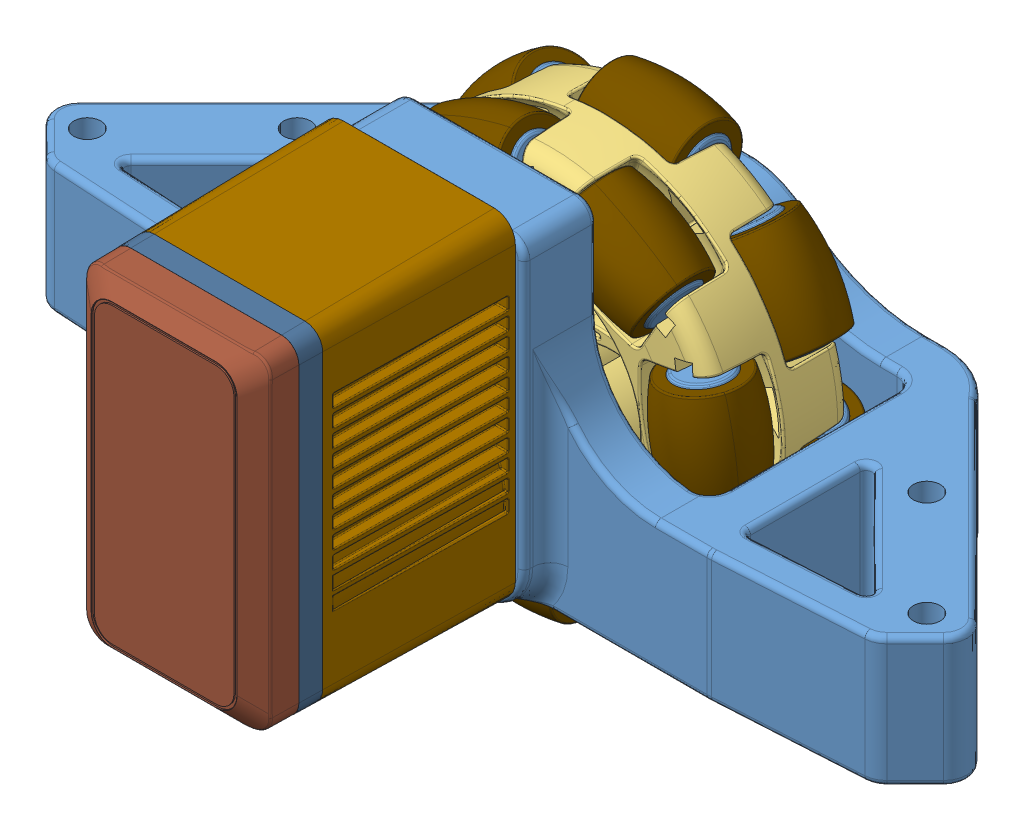
SolidWorks assembly holo_bracket_v4_testfit, configuration Default. Lengths in mm.
Overall size (155.99 97.03 100.21).
88 component instances, 22 part files, 14 mates.
Components (placement in the parent):
- holo_bracket_v4-1: holo_bracket_v4 [Default] at (53.3418 73.7776 128.0643) size (155.99 57.17 55.6)
- V5 Smart Motor (276-4840) no cap-1: V5 Smart Motor (276-4840) no cap [Default] at (53.3418 105.5276 175.3143) x (0 -1 0) z (0 0 -1) size (59.01 35.33 59.91)
  - V5 Smart Motor (276-4840).step-1: V5 Smart Motor (276-4840).step [Default] at origin size (59.01 35.33 59.91)
    - 276-4840-900 Rev6_Instruction.step-1: 276-4840-900 Rev6_Instruction.step [Default] at (-14.3 0 -17.2) size (52.79 15.94 38.15)
      - 276-4840-901 Rev6.step-1: 276-4840-901 Rev6.step [Default] at (10.75 -10.05 17.8) x (-1 0 0) z (0 0 1) size (49.9 1.6 38.15)
      - 276-4840-902 Rev2.step-1: 276-4840-902 Rev2.step [Default] at (31.25 -9.25 6.2) x (0 0 -1) z (0 -1 0) size (10.35 11.39 15.94)
      - 276-4840-022 Rev4.step-1: 276-4840-022 Rev4.step [Default] at (31.25 -9.25 6.2) x (0 0 -1) z (1 0 0) size (10.26 9.1 5.51)
    - 276-4840-110 Rev10_Instruction.step-1: 276-4840-110 Rev10_Instruction.step [Default] at (12.7 0 14.7) size (35.33 35.33 31.1)
      - 276-4840-061 Rev7_Ring_Gear_Fixed01 .6 Rev3.step-1: 276-4840-061 Rev7_Ring_Gear_Fixed01 .6 Rev3.step [Default] at origin size (28.79 28.39 24.6)
      - 276-4840-018 Rev6.step-1: 276-4840-018 Rev6.step [Default] at (0 0 6.7) x (-0.483174 0.875524 0) z (0 0 1) size (26 26 12.3)
      - 276-4840-059 Rev2.step-1: 276-4840-059 Rev2.step [Default] at (0 0 10.3) size (28.4 28.4 8.5)
      - 276-4840-062 Rev1.step-1: 276-4840-062 Rev1.step [Default] at (-12.1353 8.8168 12.3) x (0.956835 -0.290632 0) z (-0.290632 -0.956835 0) size (3.2 6.56 3.2)
      - 276-4840-062 Rev1.step-2: 276-4840-062 Rev1.step [Default] at (12.1353 8.8168 12.3) x (0.978427 0.206591 0) z (0.206591 -0.978427 0) size (3.2 6.56 3.2)
      - 276-4840-062 Rev1.step-3: 276-4840-062 Rev1.step [Default] at (-12.1353 -8.8168 12.3) x (0.72563 0.688086 0) z (0.688086 -0.72563 0) size (3.2 6.56 3.2)
    - 276-4840-001 Rev38.step-1: 276-4840-001 Rev38.step [Default] at origin size (57.3 33 46.9)
    - 276-4840-005 Rev27.step-1: 276-4840-005 Rev27.step [Default] at (0 0 -17.95) size (56.17 31.87 12.9)
    - 276-4840-004 Rev16.step-1: 276-4840-004 Rev16.step [Default] at (0 0 -19.2) size (56.01 31.71 9.21)
    - 276-4840-009 Rev3.step-1: 276-4840-009 Rev3.step [Default] at (25.45 13.5 15.7) x (0.19987 -0.979823 0) z (-0.979823 -0.19987 0) size (3.4 41.31 4.34)
    - 276-4840-009 Rev3.step-2: 276-4840-009 Rev3.step [Default] at (-25.45 -13.5 15.7) x (-0.998855 0.047836 0) z (0.047836 0.998855 0) size (3.4 41.31 4.34)
    - 276-4840-009 Rev3.step-3: 276-4840-009 Rev3.step [Default] at (25.45 -13.5 15.7) x (-0.975374 0.220559 0) z (0.220559 0.975374 0) size (3.4 41.31 4.34)
    - 276-4840-009 Rev3.step-4: 276-4840-009 Rev3.step [Default] at (-25.45 13.5 15.7) x (-0.922256 0.38658 0) z (0.38658 0.922256 0) size (3.4 41.31 4.34)
    - 276-4840-025 Rev19.step-1: 276-4840-025 Rev19.step [Default] at (12.7 0 -22.63) x (-0.993315 0.115437 0) z (0 0 1) size (14.82 14.83 35.18)
- 0.375_ ID x 0.875_ OD x 0.281_ WD (Radial Bearing) (217-3239)-1: 0.375_ ID x 0.875_ OD x 0.281_ WD (Radial Bearing) (217-3239) [Default] at (53.3418 92.8276 103.3769) x (0 0 1) z (-1 0 0) size (7.14 22.23 22.23)
- 0.375in_ID_Bearing_Insert-1: 0.375in_ID_Bearing_Insert [Default] at (53.3418 92.8276 110.5143) x (-0.838817 0.544413 0) z (0 0 -1) size (9.4 9.4 7.14)
- Drive Shaft 2in-1: Drive Shaft 2in [Default] at (53.3418 92.8276 1.1143) x (-0.544413 -0.838817 0) z (0 0 1) size (3.28 3.28 50.8)
- Shaft Collar (276-2010)-1: Shaft Collar (276-2010) [Default] at (53.3418 92.8276 113.8163) size (11 11.35 6.6)
- 2.75 Omni with inserts (276-1902) -1: 2.75 Omni with inserts (276-1902)  [Default] at (0.1559 110.7488 59.7876) x (0.152128 -0.988361 0) z (0 0 1) size (87.15 87.98 47.75)
  - 2.75 Omni-Directional Wheel - Double Roller (276-1902) -1: 2.75 Omni-Directional Wheel - Double Roller (276-1902)  [Default] at (25.8037 49.8406 68.5807) size (87.15 87.98 47.75)
    - 2.75 Omni-Directional Wheel - Double Roller (276-1902) .step-1: 2.75 Omni-Directional Wheel - Double Roller (276-1902) .step [Default] at origin size (87.15 87.98 47.75)
      - 276-1902-010 Rev1.step-1: 276-1902-010 Rev1.step [Default] at (0 27.5 8) x (1 0 0) z (0 0.828233 0.560383) size (23 27.81 20.35)
        - 276-1902-011 Rev1.step-1: 276-1902-011 Rev1.step [Default] at (0 -6.325 -26.7627) x (1 0 0) z (0 -0.973191 0.23) size (16.5 15 25.03)
        - 276-1902-012 Rev1.step-1: 276-1902-012 Rev1.step [Default] at origin size (17.5 10.34 18.34)
        - 276-1902-003 Rev1.step-1: 276-1902-003 Rev1.step [Default] x (0 -0.928523 0.371275) z (1 0 0) size (2 2 23)
      - 276-1902-010 Rev1.step-2: 276-1902-010 Rev1.step [Default] at (0 -27.5 -8) x (1 0 0) z (0 0.410464 0.911877) size (23 27.81 20.35)
        - 276-1902-011 Rev1.step-1: 276-1902-011 Rev1.step [Default] at (0 -6.325 -26.7627) x (1 0 0) z (0 -0.973191 0.23) size (16.5 15 25.03)
        - 276-1902-012 Rev1.step-1: 276-1902-012 Rev1.step [Default] at origin size (17.5 10.34 18.34)
        - 276-1902-003 Rev1.step-1: 276-1902-003 Rev1.step [Default] x (0 -0.928523 0.371275) z (1 0 0) size (2 2 23)
      - 276-1902-010 Rev1.step-3: 276-1902-010 Rev1.step [Default] at (-21.5004 -17.146 -8) x (0.62349 -0.781831 0) z (0.320913 0.25592 0.911877) size (23 27.81 20.35)
        - 276-1902-011 Rev1.step-1: 276-1902-011 Rev1.step [Default] at (0 -6.325 -26.7627) x (1 0 0) z (0 -0.973191 0.23) size (16.5 15 25.03)
        - 276-1902-012 Rev1.step-1: 276-1902-012 Rev1.step [Default] at origin size (17.5 10.34 18.34)
        - 276-1902-003 Rev1.step-1: 276-1902-003 Rev1.step [Default] x (0 -0.928523 0.371275) z (1 0 0) size (2 2 23)
      - 276-1902-010 Rev1.step-4: 276-1902-010 Rev1.step [Default] at (-26.8105 6.1193 -8) x (-0.222521 -0.974928 0) z (0.400172 -0.091337 0.911877) size (23 27.81 20.35)
        - 276-1902-011 Rev1.step-1: 276-1902-011 Rev1.step [Default] at (0 -6.325 -26.7627) x (1 0 0) z (0 -0.973191 0.23) size (16.5 15 25.03)
        - 276-1902-012 Rev1.step-1: 276-1902-012 Rev1.step [Default] at origin size (17.5 10.34 18.34)
        - 276-1902-003 Rev1.step-1: 276-1902-003 Rev1.step [Default] x (0 -0.928523 0.371275) z (1 0 0) size (2 2 23)
      - 276-1902-010 Rev1.step-5: 276-1902-010 Rev1.step [Default] at (-11.9318 24.7766 -8) x (-0.900969 -0.433884 0) z (0.178093 -0.369815 0.911877) size (23 27.81 20.35)
        - 276-1902-011 Rev1.step-1: 276-1902-011 Rev1.step [Default] at (0 -6.325 -26.7627) x (1 0 0) z (0 -0.973191 0.23) size (16.5 15 25.03)
        - 276-1902-012 Rev1.step-1: 276-1902-012 Rev1.step [Default] at origin size (17.5 10.34 18.34)
        - 276-1902-003 Rev1.step-1: 276-1902-003 Rev1.step [Default] x (0 -0.928523 0.371275) z (1 0 0) size (2 2 23)
      - 276-1902-010 Rev1.step-6: 276-1902-010 Rev1.step [Default] at (11.9318 24.7766 -8) x (-0.900969 0.433884 0) z (-0.178093 -0.369815 0.911877) size (23 27.81 20.35)
        - 276-1902-011 Rev1.step-1: 276-1902-011 Rev1.step [Default] at (0 -6.325 -26.7627) x (1 0 0) z (0 -0.973191 0.23) size (16.5 15 25.03)
        - 276-1902-012 Rev1.step-1: 276-1902-012 Rev1.step [Default] at origin size (17.5 10.34 18.34)
        - 276-1902-003 Rev1.step-1: 276-1902-003 Rev1.step [Default] x (0 -0.928523 0.371275) z (1 0 0) size (2 2 23)
      - 276-1902-010 Rev1.step-7: 276-1902-010 Rev1.step [Default] at (26.8105 6.1193 -8) x (-0.222521 0.974928 0) z (-0.400172 -0.091337 0.911877) size (23 27.81 20.35)
        - 276-1902-011 Rev1.step-1: 276-1902-011 Rev1.step [Default] at (0 -6.325 -26.7627) x (1 0 0) z (0 -0.973191 0.23) size (16.5 15 25.03)
        - 276-1902-012 Rev1.step-1: 276-1902-012 Rev1.step [Default] at origin size (17.5 10.34 18.34)
        - 276-1902-003 Rev1.step-1: 276-1902-003 Rev1.step [Default] x (0 -0.928523 0.371275) z (1 0 0) size (2 2 23)
      - 276-1902-010 Rev1.step-8: 276-1902-010 Rev1.step [Default] at (21.5004 -17.146 -8) x (0.62349 0.781831 0) z (-0.320913 0.25592 0.911877) size (23 27.81 20.35)
        - 276-1902-011 Rev1.step-1: 276-1902-011 Rev1.step [Default] at (0 -6.325 -26.7627) x (1 0 0) z (0 -0.973191 0.23) size (16.5 15 25.03)
        - 276-1902-012 Rev1.step-1: 276-1902-012 Rev1.step [Default] at origin size (17.5 10.34 18.34)
        - 276-1902-003 Rev1.step-1: 276-1902-003 Rev1.step [Default] x (0 -0.928523 0.371275) z (1 0 0) size (2 2 23)
      - 276-1902-010 Rev1.step-9: 276-1902-010 Rev1.step [Default] at (21.5004 17.146 8) x (0.62349 -0.781831 0) z (0.647539 0.516395 0.560383) size (23 27.81 20.35)
        - 276-1902-011 Rev1.step-1: 276-1902-011 Rev1.step [Default] at (0 -6.325 -26.7627) x (1 0 0) z (0 -0.973191 0.23) size (16.5 15 25.03)
        - 276-1902-012 Rev1.step-1: 276-1902-012 Rev1.step [Default] at origin size (17.5 10.34 18.34)
        - 276-1902-003 Rev1.step-1: 276-1902-003 Rev1.step [Default] x (0 -0.928523 0.371275) z (1 0 0) size (2 2 23)
      - 276-1902-010 Rev1.step-10: 276-1902-010 Rev1.step [Default] at (26.8105 -6.1193 8) x (-0.222521 -0.974928 0) z (0.807468 -0.184299 0.560383) size (23 27.81 20.35)
        - 276-1902-011 Rev1.step-1: 276-1902-011 Rev1.step [Default] at (0 -6.325 -26.7627) x (1 0 0) z (0 -0.973191 0.23) size (16.5 15 25.03)
        - 276-1902-012 Rev1.step-1: 276-1902-012 Rev1.step [Default] at origin size (17.5 10.34 18.34)
        - 276-1902-003 Rev1.step-1: 276-1902-003 Rev1.step [Default] x (0 -0.928523 0.371275) z (1 0 0) size (2 2 23)
      - 276-1902-010 Rev1.step-11: 276-1902-010 Rev1.step [Default] at (11.9318 -24.7766 8) x (-0.900969 -0.433884 0) z (0.359357 -0.746212 0.560383) size (23 27.81 20.35)
        - 276-1902-011 Rev1.step-1: 276-1902-011 Rev1.step [Default] at (0 -6.325 -26.7627) x (1 0 0) z (0 -0.973191 0.23) size (16.5 15 25.03)
        - 276-1902-012 Rev1.step-1: 276-1902-012 Rev1.step [Default] at origin size (17.5 10.34 18.34)
        - 276-1902-003 Rev1.step-1: 276-1902-003 Rev1.step [Default] x (0 -0.928523 0.371275) z (1 0 0) size (2 2 23)
      - 276-1902-010 Rev1.step-12: 276-1902-010 Rev1.step [Default] at (-11.9318 -24.7766 8) x (-0.900969 0.433884 0) z (-0.359357 -0.746212 0.560383) size (23 27.81 20.35)
        - 276-1902-011 Rev1.step-1: 276-1902-011 Rev1.step [Default] at (0 -6.325 -26.7627) x (1 0 0) z (0 -0.973191 0.23) size (16.5 15 25.03)
        - 276-1902-012 Rev1.step-1: 276-1902-012 Rev1.step [Default] at origin size (17.5 10.34 18.34)
        - 276-1902-003 Rev1.step-1: 276-1902-003 Rev1.step [Default] x (0 -0.928523 0.371275) z (1 0 0) size (2 2 23)
      - 276-1902-010 Rev1.step-13: 276-1902-010 Rev1.step [Default] at (-26.8105 -6.1193 8) x (-0.222521 0.974928 0) z (-0.807468 -0.184299 0.560383) size (23 27.81 20.35)
        - 276-1902-011 Rev1.step-1: 276-1902-011 Rev1.step [Default] at (0 -6.325 -26.7627) x (1 0 0) z (0 -0.973191 0.23) size (16.5 15 25.03)
        - 276-1902-012 Rev1.step-1: 276-1902-012 Rev1.step [Default] at origin size (17.5 10.34 18.34)
        - 276-1902-003 Rev1.step-1: 276-1902-003 Rev1.step [Default] x (0 -0.928523 0.371275) z (1 0 0) size (2 2 23)
      - 276-1902-010 Rev1.step-14: 276-1902-010 Rev1.step [Default] at (-21.5004 17.146 8) x (0.62349 0.781831 0) z (-0.647539 0.516395 0.560383) size (23 27.81 20.35)
        - 276-1902-011 Rev1.step-1: 276-1902-011 Rev1.step [Default] at (0 -6.325 -26.7627) x (1 0 0) z (0 -0.973191 0.23) size (16.5 15 25.03)
        - 276-1902-012 Rev1.step-1: 276-1902-012 Rev1.step [Default] at origin size (17.5 10.34 18.34)
        - 276-1902-003 Rev1.step-1: 276-1902-003 Rev1.step [Default] x (0 -0.928523 0.371275) z (1 0 0) size (2 2 23)
      - 276-1902-002 Rev3.step-1: 276-1902-002 Rev3.step [Default] at origin size (66.55 66.02 25.07)
  - Metal Shaft Inserts (276-3881-002)-1: Metal Shaft Inserts (276-3881-002) [Default] at (25.8037 49.8406 79.8307) x (0 -1 0) z (1 0 0) size (10.03 5.08 10.03)
  - Metal Shaft Inserts (276-3881-002)-2: Metal Shaft Inserts (276-3881-002) [Default] at (25.8037 49.8406 57.3307) x (1 0 0) z (0 -1 0) size (10.03 5.08 10.03)
Mates (geometry in assembly coordinates):
- Concentric1: concentric aligned: cylinder of holo_bracket_v4-1 through (53.3418 92.8276 102.5133) axis (0 0 1) radius 14.5; cone of V5 Smart Motor (276-4840) no cap-1/V5 Smart Motor (276-4840).step-1/276-4840-110 Rev10_Instruction.step-1/276-4840-061 Rev7_Ring_Gear_Fixed01 .6 Rev3.step-1 through (53.3418 92.8276 172.9143) axis (0 0 1)
- Coincident1: coincident anti-aligned: plane of holo_bracket_v4-1 through (53.3418 73.7776 158.1143) normal (0 0 1); plane of V5 Smart Motor (276-4840) no cap-1/V5 Smart Motor (276-4840).step-1/276-4840-001 Rev38.step-1 through (40.4418 130.5776 158.1143) normal (0 0 -1)
- Parallel1: parallel aligned: line of holo_bracket_v4-1 through (39.3418 130.4776 157.1143) axis (1 0 0); line of V5 Smart Motor (276-4840) no cap-1/V5 Smart Motor (276-4840).step-1/276-4840-001 Rev38.step-1 through (40.4418 134.1776 159.1143) axis (1 0 0)
- Concentric2: concentric anti-aligned: cylinder of 0.375_ ID x 0.875_ OD x 0.281_ WD (Radial Bearing) (217-3239)-1 through (53.3418 92.8276 88.84) axis (0 0 -1) radius 4.763; cylinder of 0.375in_ID_Bearing_Insert-1 through (53.3418 92.8276 103.3769) axis (0 0 1) radius 4.7
- Coincident2: coincident aligned: plane of 0.375_ ID x 0.875_ OD x 0.281_ WD (Radial Bearing) (217-3239)-1 through (53.3418 87.6646 103.3769) normal (0 0 -1); plane of 0.375in_ID_Bearing_Insert-1 through (53.3418 92.8276 103.3769) normal (0 0 -1)
- Concentric3: concentric anti-aligned: cylinder of holo_bracket_v4-1 through (53.3418 92.8276 103.3769) axis (0 0 1) radius 11.25; cylinder of 0.375_ ID x 0.875_ OD x 0.281_ WD (Radial Bearing) (217-3239)-1 through (53.3418 92.8276 88.84) axis (0 0 -1) radius 11.113
- Coincident3: coincident anti-aligned: plane of holo_bracket_v4-1 through (53.3418 92.8276 103.3769) normal (0 0 1); plane of 0.375_ ID x 0.875_ OD x 0.281_ WD (Radial Bearing) (217-3239)-1 through (53.3418 83.3446 103.3769) normal (0 0 -1)
- Concentric4: concentric aligned: circle of 0.375in_ID_Bearing_Insert-1; circle of Drive Shaft 2in-1
- Parallel2: parallel aligned: plane of 0.375in_ID_Bearing_Insert-1 through (51.1342 92.1741 103.3769) normal (0.544413 0.838817 0); plane of Drive Shaft 2in-1 through (52.8744 95.0234 153.5143) normal (0.544413 0.838817 0)
- Coincident7: coincident anti-aligned: plane of V5 Smart Motor (276-4840) no cap-1/V5 Smart Motor (276-4840).step-1/276-4840-110 Rev10_Instruction.step-1/276-4840-018 Rev6.step-1 through (53.3418 92.8276 153.5143) normal (0 0 -1); plane of Drive Shaft 2in-1 through (55.5377 93.2949 153.5143) normal (0 0 1)
- Coincident8: coincident anti-aligned: plane of 0.375in_ID_Bearing_Insert-1 through (53.3418 92.8276 110.5143) normal (0 0 1); plane of Shaft Collar (276-2010)-1 through (53.3418 92.8276 110.5143) normal (0 0 -1)
- Concentric5: concentric anti-aligned: circle of 0.375in_ID_Bearing_Insert-1; circle of Shaft Collar (276-2010)-1
- Concentric6: concentric aligned: circle of Shaft Collar (276-2010)-1; circle of 2.75 Omni with inserts (276-1902) -1/Metal Shaft Inserts (276-3881-002)-1
- Coincident9: coincident anti-aligned: plane of Shaft Collar (276-2010)-1 through (53.3418 92.8276 117.1183) normal (0 0 1); plane of 2.75 Omni with inserts (276-1902) -1/Metal Shaft Inserts (276-3881-002)-2 through (53.3418 92.8276 117.1183) normal (0 0 -1)
